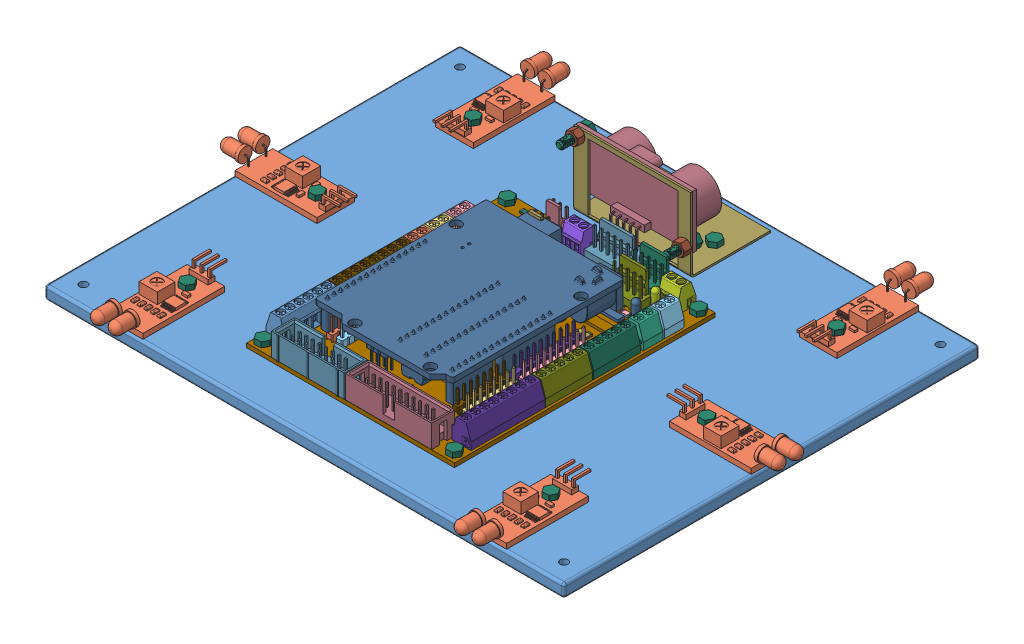
SolidWorks assembly upper assembly, configuration Default. Lengths in mm.
Overall size (215.6 59.56 175.6).
233 component instances, 198 part files, 38 mates.
Components (placement in the parent):
- base-1: base [Default] at (100.7293 111.0554 133.5181) size (200 5 160)
- Infrared Sensor (2)-1: Infrared Sensor (2) [Default] at (30.7293 116.0554 197.1202) x (-1 0 0) z (0 0 -1) size (14.5 8.55 44.7)
- Arduino Uno shield with Unokk-1: Arduino Uno shield with Unokk [Standard] at (60.7243 116.0554 95.3431) x (0 0 1) z (0 1 0) size (100.65 90.35 23.92)
  - PPP5f08ec48b7509.stp-1: PPP5f08ec48b7509.stp [Standard] at origin size (100.65 80.01 15.26)
    - CAPRR500W50L750T250H650P002.stp-1: CAPRR500W50L750T250H650P002.stp [Standard] at (21.59 34.29 1.57) x (0 -1 0) z (0 0 1) size (7.5 2.5 6.5)
    - CAPRR500W50L750T250H650P001.stp-1: CAPRR500W50L750T250H650P001.stp [Standard] at (21.59 34.29 1.57) x (0 -1 0) z (0 0 1) size (0.5 0.5 6.5)
    - CAPRR500W50L750T250H650P.stp-1: CAPRR500W50L750T250H650P.stp [Standard] at (21.59 34.29 1.57) x (0 -1 0) z (0 0 1) size (0.5 0.5 6.5)
    - CAPRR500W50L750T250H650P003.stp-1: CAPRR500W50L750T250H650P003.stp [Standard] at (20.32 26.67 1.57) x (0 -1 0) z (0 0 1) size (7.5 2.5 6.5)
    - CAPRR500W50L750T250H650P004.stp-1: CAPRR500W50L750T250H650P004.stp [Standard] at (20.32 26.67 1.57) x (0 -1 0) z (0 0 1) size (0.5 0.5 6.5)
    - CAPRR500W50L750T250H650P005.stp-1: CAPRR500W50L750T250H650P005.stp [Standard] at (20.32 26.67 1.57) x (0 -1 0) z (0 0 1) size (0.5 0.5 6.5)
    - Component_1.stp-1: Component_1.stp [Standard] at (26.67 60.325 1.57) x (0 1 0) z (0 0 1) size (15.24 3.56 1)
    - SW3dPS-MELF_Cylinder5.stp-1: SW3dPS-MELF_Cylinder5.stp [Standard] at (33.02 13.208 1.57) x (0 1 0) z (0 0 1) size (0.5 2.5 2.5)
    - SW3dPS-MELF_Cylinder7.stp-1: SW3dPS-MELF_Cylinder7.stp [Standard] at (33.02 13.208 1.57) x (0 1 0) z (0 0 1) size (0.8 2.5 2.5)
    - SW3dPS-MELF_Board1.stp-1: SW3dPS-MELF_Board1.stp [Standard] at (33.02 13.208 1.57) x (0 1 0) z (0 0 1) size (1.7 0.01 0.01)
    - SW3dPS-MELF_Cylinder9.stp-1: SW3dPS-MELF_Cylinder9.stp [Standard] at (33.02 13.208 1.57) x (0 1 0) z (0 0 1) size (2.4 2.5 2.5)
    - SW3dPS-MELF_Cylinder8.stp-1: SW3dPS-MELF_Cylinder8.stp [Standard] at (33.02 13.208 1.57) x (0 1 0) z (0 0 1) size (0.5 2.5 2.5)
    - SW3dPS-MELF_Cylinder6.stp-1: SW3dPS-MELF_Cylinder6.stp [Standard] at (33.02 13.208 1.57) x (0 1 0) z (0 0 1) size (0.8 2.5 2.5)
    - SW3dPS-MELF_Cylinder010.stp-1: SW3dPS-MELF_Cylinder010.stp [Standard] at (41.275 13.208 1.57) x (0 1 0) z (0 0 1) size (0.5 2.5 2.5)
    - SW3dPS-MELF_Cylinder011.stp-1: SW3dPS-MELF_Cylinder011.stp [Standard] at (41.275 13.208 1.57) x (0 1 0) z (0 0 1) size (0.8 2.5 2.5)
    - SW3dPS-MELF_Board002.stp-1: SW3dPS-MELF_Board002.stp [Standard] at (41.275 13.208 1.57) x (0 1 0) z (0 0 1) size (1.7 0.01 0.01)
    - SW3dPS-MELF_Cylinder012.stp-1: SW3dPS-MELF_Cylinder012.stp [Standard] at (41.275 13.208 1.57) x (0 1 0) z (0 0 1) size (2.4 2.5 2.5)
    - SW3dPS-MELF_Cylinder013.stp-1: SW3dPS-MELF_Cylinder013.stp [Standard] at (41.275 13.208 1.57) x (0 1 0) z (0 0 1) size (0.5 2.5 2.5)
    - SW3dPS-MELF_Cylinder014.stp-1: SW3dPS-MELF_Cylinder014.stp [Standard] at (41.275 13.208 1.57) x (0 1 0) z (0 0 1) size (0.8 2.5 2.5)
    - SW3dPS-MELF_Cylinder015.stp-1: SW3dPS-MELF_Cylinder015.stp [Standard] at (24.765 13.208 1.57) x (0 1 0) z (0 0 1) size (0.5 2.5 2.5)
    - SW3dPS-MELF_Cylinder016.stp-1: SW3dPS-MELF_Cylinder016.stp [Standard] at (24.765 13.208 1.57) x (0 1 0) z (0 0 1) size (0.8 2.5 2.5)
    - SW3dPS-MELF_Board003.stp-1: SW3dPS-MELF_Board003.stp [Standard] at (24.765 13.208 1.57) x (0 1 0) z (0 0 1) size (1.7 0.01 0.01)
    - SW3dPS-MELF_Cylinder017.stp-1: SW3dPS-MELF_Cylinder017.stp [Standard] at (24.765 13.208 1.57) x (0 1 0) z (0 0 1) size (2.4 2.5 2.5)
    - SW3dPS-MELF_Cylinder018.stp-1: SW3dPS-MELF_Cylinder018.stp [Standard] at (24.765 13.208 1.57) x (0 1 0) z (0 0 1) size (0.5 2.5 2.5)
    - SW3dPS-MELF_Cylinder019.stp-1: SW3dPS-MELF_Cylinder019.stp [Standard] at (24.765 13.208 1.57) x (0 1 0) z (0 0 1) size (0.8 2.5 2.5)
    - Component_2.stp-1: Component_2.stp [Standard] at (20.955 59.69 1.57) x (0 -1 0) z (0 0 1) size (10.16 2.54 1)
    - Component_3.stp-1: Component_3.stp [Standard] at (20.32 43.815 1.57) x (-1 0 0) z (0 0 1) size (10.16 3.17 1)
    - =_[0_1_1_2].stp-1: =_[0_1_1_2].stp [Standard] at (10.795 24.13 1.57) x (0 -1 0) z (0 0 1) size (7.62 5.8 15.26)
    - =_[0_1_1_2]001.stp-1: =_[0_1_1_2]001.stp [Standard] at (3.81 24.13 1.57) x (0 -1 0) z (0 0 1) size (7.62 5.8 15.26)
    - =_[0_1_1_2]002.stp-1: =_[0_1_1_2]002.stp [Standard] at (4.445 44.45 1.57) x (0 1 0) z (0 0 1) size (15.24 5.8 15.26)
    - =_[0_1_1_2]003.stp-1: =_[0_1_1_2]003.stp [Standard] at (4.699 59.055 1.57) x (0 1 0) z (0 0 1) size (12.7 5.8 15.26)
    - =_[0_1_1_2]004.stp-1: =_[0_1_1_2]004.stp [Standard] at (12.7 59.055 1.57) x (0 1 0) z (0 0 1) size (12.7 5.8 15.26)
    - 1.stp-1: 1.stp [Standard] at (49.276 63.5 1.57) x (-1 0 0) z (0 0 1) size (25.4 2.5 11.2)
    - 1001.stp-1: 1001.stp [Standard] at (73.66 63.5 1.57) x (-1 0 0) z (0 0 1) size (20.32 2.5 11.2)
    - 1002.stp-1: 1002.stp [Standard] at (55.88 15.24 1.57) x (-1 0 0) z (0 0 1) size (20.32 2.5 11.2)
    - 1003.stp-1: 1003.stp [Standard] at (76.2 15.24 1.57) size (15.24 2.5 11.2)
    - 1004.stp-1: 1004.stp [Standard] at (73.66 67.31 1.57) x (-1 0 0) z (0 0 1) size (20.32 2.5 11.2)
    - 1005.stp-1: 1005.stp [Standard] at (49.276 67.31 1.57) x (-1 0 0) z (0 0 1) size (25.4 2.5 11.2)
    - 1006.stp-1: 1006.stp [Standard] at (76.2 19.05 1.57) size (15.24 2.5 11.2)
    - 1007.stp-1: 1007.stp [Standard] at (55.88 19.05 1.57) x (-1 0 0) z (0 0 1) size (20.32 2.5 11.2)
    - LEDRD254W000D310H620P002.stp-1: LEDRD254W000D310H620P002.stp [Standard] at (12.065 69.215 1.57) x (0 1 0) z (0 0 1) size (3.1 3.1 6.2)
    - LEDRD254W000D310H620P.stp-1: LEDRD254W000D310H620P.stp [Standard] at (12.065 69.215 1.57) x (0 1 0) z (0 0 1) size (0.38 0.38 6.2)
    - LEDRD254W000D310H620P001.stp-1: LEDRD254W000D310H620P001.stp [Standard] at (12.065 69.215 1.57) x (0 1 0) z (0 0 1) size (0.38 0.38 6.2)
    - LEDRD254W000D310H620P003.stp-1: LEDRD254W000D310H620P003.stp [Standard] at (19.685 69.215 1.57) x (0 1 0) z (0 0 1) size (3.1 3.1 6.2)
    - LEDRD254W000D310H620P004.stp-1: LEDRD254W000D310H620P004.stp [Standard] at (19.685 69.215 1.57) x (0 1 0) z (0 0 1) size (0.38 0.38 6.2)
    - LEDRD254W000D310H620P005.stp-1: LEDRD254W000D310H620P005.stp [Standard] at (19.685 69.215 1.57) x (0 1 0) z (0 0 1) size (0.38 0.38 6.2)
    - LEDRD254W000D310H620P006.stp-1: LEDRD254W000D310H620P006.stp [Standard] at (50.8 52.705 1.57) x (-1 0 0) z (0 0 1) size (3.1 3.1 6.2)
    - LEDRD254W000D310H620P007.stp-1: LEDRD254W000D310H620P007.stp [Standard] at (50.8 52.705 1.57) x (-1 0 0) z (0 0 1) size (0.38 0.38 6.2)
    - LEDRD254W000D310H620P008.stp-1: LEDRD254W000D310H620P008.stp [Standard] at (50.8 52.705 1.57) x (-1 0 0) z (0 0 1) size (0.38 0.38 6.2)
    - LEDRD254W000D310H620P009.stp-1: LEDRD254W000D310H620P009.stp [Standard] at (45.72 52.705 1.57) x (-1 0 0) z (0 0 1) size (3.1 3.1 6.2)
    - LEDRD254W000D310H620P010.stp-1: LEDRD254W000D310H620P010.stp [Standard] at (45.72 52.705 1.57) x (-1 0 0) z (0 0 1) size (0.38 0.38 6.2)
    - LEDRD254W000D310H620P011.stp-1: LEDRD254W000D310H620P011.stp [Standard] at (45.72 52.705 1.57) x (-1 0 0) z (0 0 1) size (0.38 0.38 6.2)
    - User_Library-TO263-3New_Extruded_2.stp-1: User_Library-TO263-3New_Extruded_2.stp [Standard] at (41.91 31.75 1.57) x (-1 0 0) z (0 0 1) size (1.4 1.53 0.51)
    - User_Library-TO263-3New_Extruded.stp-1: User_Library-TO263-3New_Extruded.stp [Standard] at (41.91 31.75 1.57) x (-1 0 0) z (0 0 1) size (1 5.77 3.36)
    - User_Library-TO263-3New_D2PACK.stp-1: User_Library-TO263-3New_D2PACK.stp [Standard] at (41.91 31.75 1.57) x (-1 0 0) z (0 0 1) size (10.41 15.85 4.61)
    - User_Library-TO263-3New_Extruded_003.stp-1: User_Library-TO263-3New_Extruded_003.stp [Standard] at (54.61 31.75 1.57) x (-1 0 0) z (0 0 1) size (1.4 1.53 0.51)
    - User_Library-TO263-3New_Extruded001.stp-1: User_Library-TO263-3New_Extruded001.stp [Standard] at (54.61 31.75 1.57) x (-1 0 0) z (0 0 1) size (1 5.77 3.36)
    - User_Library-TO263-3New_D2PACK001.stp-1: User_Library-TO263-3New_D2PACK001.stp [Standard] at (54.61 31.75 1.57) x (-1 0 0) z (0 0 1) size (10.41 15.85 4.61)
    - User_Library-TO263-3New_Extruded_004.stp-1: User_Library-TO263-3New_Extruded_004.stp [Standard] at (29.21 31.75 1.57) x (-1 0 0) z (0 0 1) size (1.4 1.53 0.51)
    - User_Library-TO263-3New_Extruded002.stp-1: User_Library-TO263-3New_Extruded002.stp [Standard] at (29.21 31.75 1.57) x (-1 0 0) z (0 0 1) size (1 5.77 3.36)
    - User_Library-TO263-3New_D2PACK002.stp-1: User_Library-TO263-3New_D2PACK002.stp [Standard] at (29.21 31.75 1.57) x (-1 0 0) z (0 0 1) size (10.41 15.85 4.61)
    - RESC3216X078.stp-1: RESC3216X078.stp [Standard] at (54.483 46.482 1.57) size (2.12 1.6 0.1)
    - RESC3216X079.stp-1: RESC3216X079.stp [Standard] at (54.483 46.482 1.57) size (3.06 1.6 0.56)
    - RESC3216X077.stp-1: RESC3216X077.stp [Standard] at (54.483 46.482 1.57) size (0.57 1.6 0.76)
    - RESC3216X080.stp-1: RESC3216X080.stp [Standard] at (54.483 46.482 1.57) size (2.12 1.6 0.1)
    - RESC3216X76.stp-1: RESC3216X76.stp [Standard] at (54.483 46.482 1.57) size (0.57 1.6 0.76)
    - RESC3216X081.stp-1: RESC3216X081.stp [Standard] at (41.91 46.355 1.57) size (2.12 1.6 0.1)
    - RESC3216X082.stp-1: RESC3216X082.stp [Standard] at (41.91 46.355 1.57) size (3.06 1.6 0.56)
    - RESC3216X083.stp-1: RESC3216X083.stp [Standard] at (41.91 46.355 1.57) size (0.57 1.6 0.76)
    - RESC3216X084.stp-1: RESC3216X084.stp [Standard] at (41.91 46.355 1.57) size (2.12 1.6 0.1)
    - RESC3216X085.stp-1: RESC3216X085.stp [Standard] at (41.91 46.355 1.57) size (0.57 1.6 0.76)
    - RESC3216X086.stp-1: RESC3216X086.stp [Standard] at (29.21 48.895 1.57) size (2.12 1.6 0.1)
    - RESC3216X087.stp-1: RESC3216X087.stp [Standard] at (29.21 48.895 1.57) size (3.06 1.6 0.56)
    - RESC3216X088.stp-1: RESC3216X088.stp [Standard] at (29.21 48.895 1.57) size (0.57 1.6 0.76)
    - RESC3216X089.stp-1: RESC3216X089.stp [Standard] at (29.21 48.895 1.57) size (2.12 1.6 0.1)
    - RESC3216X090.stp-1: RESC3216X090.stp [Standard] at (29.21 48.895 1.57) size (0.57 1.6 0.76)
    - RESC3216X091.stp-1: RESC3216X091.stp [Standard] at (33.02 60.96 1.57) size (2.12 1.6 0.1)
    - RESC3216X092.stp-1: RESC3216X092.stp [Standard] at (33.02 60.96 1.57) size (3.06 1.6 0.56)
    - RESC3216X093.stp-1: RESC3216X093.stp [Standard] at (33.02 60.96 1.57) size (0.57 1.6 0.76)
    - RESC3216X094.stp-1: RESC3216X094.stp [Standard] at (33.02 60.96 1.57) size (2.12 1.6 0.1)
    - RESC3216X095.stp-1: RESC3216X095.stp [Standard] at (33.02 60.96 1.57) size (0.57 1.6 0.76)
    - RESC3216X096.stp-1: RESC3216X096.stp [Standard] at (33.02 63.5 1.57) size (2.12 1.6 0.1)
    - RESC3216X097.stp-1: RESC3216X097.stp [Standard] at (33.02 63.5 1.57) size (3.06 1.6 0.56)
    - RESC3216X098.stp-1: RESC3216X098.stp [Standard] at (33.02 63.5 1.57) size (0.57 1.6 0.76)
    - RESC3216X099.stp-1: RESC3216X099.stp [Standard] at (33.02 63.5 1.57) size (2.12 1.6 0.1)
    - RESC3216X100.stp-1: RESC3216X100.stp [Standard] at (33.02 63.5 1.57) size (0.57 1.6 0.76)
    - RESC3216X101.stp-1: RESC3216X101.stp [Standard] at (15.875 69.215 1.57) x (0 -1 0) z (0 0 1) size (2.12 1.6 0.1)
    - RESC3216X102.stp-1: RESC3216X102.stp [Standard] at (15.875 69.215 1.57) x (0 -1 0) z (0 0 1) size (3.06 1.6 0.56)
    - RESC3216X103.stp-1: RESC3216X103.stp [Standard] at (15.875 69.215 1.57) x (0 -1 0) z (0 0 1) size (0.57 1.6 0.76)
    - RESC3216X104.stp-1: RESC3216X104.stp [Standard] at (15.875 69.215 1.57) x (0 -1 0) z (0 0 1) size (2.12 1.6 0.1)
    - RESC3216X105.stp-1: RESC3216X105.stp [Standard] at (15.875 69.215 1.57) x (0 -1 0) z (0 0 1) size (0.57 1.6 0.76)
    - RESC3216X106.stp-1: RESC3216X106.stp [Standard] at (17.907 63.627 1.57) x (0 1 0) z (0 0 1) size (2.12 1.6 0.1)
    - RESC3216X107.stp-1: RESC3216X107.stp [Standard] at (17.907 63.627 1.57) x (0 1 0) z (0 0 1) size (3.06 1.6 0.56)
    - RESC3216X108.stp-1: RESC3216X108.stp [Standard] at (17.907 63.627 1.57) x (0 1 0) z (0 0 1) size (0.57 1.6 0.76)
    - RESC3216X109.stp-1: RESC3216X109.stp [Standard] at (17.907 63.627 1.57) x (0 1 0) z (0 0 1) size (2.12 1.6 0.1)
    - RESC3216X110.stp-1: RESC3216X110.stp [Standard] at (17.907 63.627 1.57) x (0 1 0) z (0 0 1) size (0.57 1.6 0.76)
    - RESC3216X111.stp-1: RESC3216X111.stp [Standard] at (50.673 57.023 1.57) x (-1 0 0) z (0 0 1) size (2.12 1.6 0.1)
    - RESC3216X112.stp-1: RESC3216X112.stp [Standard] at (50.673 57.023 1.57) x (-1 0 0) z (0 0 1) size (3.06 1.6 0.56)
    - RESC3216X113.stp-1: RESC3216X113.stp [Standard] at (50.673 57.023 1.57) x (-1 0 0) z (0 0 1) size (0.57 1.6 0.76)
    - RESC3216X114.stp-1: RESC3216X114.stp [Standard] at (50.673 57.023 1.57) x (-1 0 0) z (0 0 1) size (2.12 1.6 0.1)
    - RESC3216X115.stp-1: RESC3216X115.stp [Standard] at (50.673 57.023 1.57) x (-1 0 0) z (0 0 1) size (0.57 1.6 0.76)
    - RESC3216X116.stp-1: RESC3216X116.stp [Standard] at (46.99 57.277 1.57) x (0 -1 0) z (0 0 1) size (2.12 1.6 0.1)
    - RESC3216X117.stp-1: RESC3216X117.stp [Standard] at (46.99 57.277 1.57) x (0 -1 0) z (0 0 1) size (3.06 1.6 0.56)
    - RESC3216X118.stp-1: RESC3216X118.stp [Standard] at (46.99 57.277 1.57) x (0 -1 0) z (0 0 1) size (0.57 1.6 0.76)
    - RESC3216X119.stp-1: RESC3216X119.stp [Standard] at (46.99 57.277 1.57) x (0 -1 0) z (0 0 1) size (2.12 1.6 0.1)
    - RESC3216X120.stp-1: RESC3216X120.stp [Standard] at (46.99 57.277 1.57) x (0 -1 0) z (0 0 1) size (0.57 1.6 0.76)
    - RESC3216X121.stp-1: RESC3216X121.stp [Standard] at (34.925 45.085 1.57) x (-1 0 0) z (0 0 1) size (2.12 1.6 0.1)
    - RESC3216X122.stp-1: RESC3216X122.stp [Standard] at (34.925 45.085 1.57) x (-1 0 0) z (0 0 1) size (3.06 1.6 0.56)
    - RESC3216X123.stp-1: RESC3216X123.stp [Standard] at (34.925 45.085 1.57) x (-1 0 0) z (0 0 1) size (0.57 1.6 0.76)
    - RESC3216X124.stp-1: RESC3216X124.stp [Standard] at (34.925 45.085 1.57) x (-1 0 0) z (0 0 1) size (2.12 1.6 0.1)
    - RESC3216X125.stp-1: RESC3216X125.stp [Standard] at (34.925 45.085 1.57) x (-1 0 0) z (0 0 1) size (0.57 1.6 0.76)
    - RESC3216X126.stp-1: RESC3216X126.stp [Standard] at (47.625 46.101 1.57) x (0 -1 0) z (0 0 1) size (2.12 1.6 0.1)
    - RESC3216X127.stp-1: RESC3216X127.stp [Standard] at (47.625 46.101 1.57) x (0 -1 0) z (0 0 1) size (3.06 1.6 0.56)
    - RESC3216X128.stp-1: RESC3216X128.stp [Standard] at (47.625 46.101 1.57) x (0 -1 0) z (0 0 1) size (0.57 1.6 0.76)
    - RESC3216X129.stp-1: RESC3216X129.stp [Standard] at (47.625 46.101 1.57) x (0 -1 0) z (0 0 1) size (2.12 1.6 0.1)
    - RESC3216X130.stp-1: RESC3216X130.stp [Standard] at (47.625 46.101 1.57) x (0 -1 0) z (0 0 1) size (0.57 1.6 0.76)
    - RESC3216X131.stp-1: RESC3216X131.stp [Standard] at (59.69 48.006 1.57) x (0 -1 0) z (0 0 1) size (2.12 1.6 0.1)
    - RESC3216X132.stp-1: RESC3216X132.stp [Standard] at (59.69 48.006 1.57) x (0 -1 0) z (0 0 1) size (3.06 1.6 0.56)
    - RESC3216X133.stp-1: RESC3216X133.stp [Standard] at (59.69 48.006 1.57) x (0 -1 0) z (0 0 1) size (0.57 1.6 0.76)
    - RESC3216X134.stp-1: RESC3216X134.stp [Standard] at (59.69 48.006 1.57) x (0 -1 0) z (0 0 1) size (2.12 1.6 0.1)
    - RESC3216X135.stp-1: RESC3216X135.stp [Standard] at (59.69 48.006 1.57) x (0 -1 0) z (0 0 1) size (0.57 1.6 0.76)
    - RESC2012X072.stp-1: RESC2012X072.stp [Standard] at (10.795 50.165 1.57) x (-1 0 0) z (0 0 1) size (1.2 1.25 0.1)
    - RESC2012X073.stp-1: RESC2012X073.stp [Standard] at (10.795 50.165 1.57) x (-1 0 0) z (0 0 1) size (1.8 1.25 0.5)
    - RESC2012X071.stp-1: RESC2012X071.stp [Standard] at (10.795 50.165 1.57) x (-1 0 0) z (0 0 1) size (0.4 1.25 0.7)
    - RESC2012X074.stp-1: RESC2012X074.stp [Standard] at (10.795 50.165 1.57) x (-1 0 0) z (0 0 1) size (1.2 1.25 0.1)
    - RESC2012X70.stp-1: RESC2012X70.stp [Standard] at (10.795 50.165 1.57) x (-1 0 0) z (0 0 1) size (0.4 1.25 0.7)
    - RESC2012X075.stp-1: RESC2012X075.stp [Standard] at (10.795 47.625 1.57) x (-1 0 0) z (0 0 1) size (1.2 1.25 0.1)
    - RESC2012X076.stp-1: RESC2012X076.stp [Standard] at (10.795 47.625 1.57) x (-1 0 0) z (0 0 1) size (1.8 1.25 0.5)
    - RESC2012X077.stp-1: RESC2012X077.stp [Standard] at (10.795 47.625 1.57) x (-1 0 0) z (0 0 1) size (0.4 1.25 0.7)
    - RESC2012X078.stp-1: RESC2012X078.stp [Standard] at (10.795 47.625 1.57) x (-1 0 0) z (0 0 1) size (1.2 1.25 0.1)
    - RESC2012X079.stp-1: RESC2012X079.stp [Standard] at (10.795 47.625 1.57) x (-1 0 0) z (0 0 1) size (0.4 1.25 0.7)
    - RESC2012X080.stp-1: RESC2012X080.stp [Standard] at (10.795 45.085 1.57) x (-1 0 0) z (0 0 1) size (1.2 1.25 0.1)
    - RESC2012X081.stp-1: RESC2012X081.stp [Standard] at (10.795 45.085 1.57) x (-1 0 0) z (0 0 1) size (1.8 1.25 0.5)
    - RESC2012X082.stp-1: RESC2012X082.stp [Standard] at (10.795 45.085 1.57) x (-1 0 0) z (0 0 1) size (0.4 1.25 0.7)
    - RESC2012X083.stp-1: RESC2012X083.stp [Standard] at (10.795 45.085 1.57) x (-1 0 0) z (0 0 1) size (1.2 1.25 0.1)
    - RESC2012X084.stp-1: RESC2012X084.stp [Standard] at (10.795 45.085 1.57) x (-1 0 0) z (0 0 1) size (0.4 1.25 0.7)
    - RESC2012X085.stp-1: RESC2012X085.stp [Standard] at (10.795 42.545 1.57) x (-1 0 0) z (0 0 1) size (1.2 1.25 0.1)
    - RESC2012X086.stp-1: RESC2012X086.stp [Standard] at (10.795 42.545 1.57) x (-1 0 0) z (0 0 1) size (1.8 1.25 0.5)
    - RESC2012X087.stp-1: RESC2012X087.stp [Standard] at (10.795 42.545 1.57) x (-1 0 0) z (0 0 1) size (0.4 1.25 0.7)
    - RESC2012X088.stp-1: RESC2012X088.stp [Standard] at (10.795 42.545 1.57) x (-1 0 0) z (0 0 1) size (1.2 1.25 0.1)
    - RESC2012X089.stp-1: RESC2012X089.stp [Standard] at (10.795 42.545 1.57) x (-1 0 0) z (0 0 1) size (0.4 1.25 0.7)
    - RESC2012X090.stp-1: RESC2012X090.stp [Standard] at (10.795 40.005 1.57) x (-1 0 0) z (0 0 1) size (1.2 1.25 0.1)
    - RESC2012X091.stp-1: RESC2012X091.stp [Standard] at (10.795 40.005 1.57) x (-1 0 0) z (0 0 1) size (1.8 1.25 0.5)
    - RESC2012X092.stp-1: RESC2012X092.stp [Standard] at (10.795 40.005 1.57) x (-1 0 0) z (0 0 1) size (0.4 1.25 0.7)
    - RESC2012X093.stp-1: RESC2012X093.stp [Standard] at (10.795 40.005 1.57) x (-1 0 0) z (0 0 1) size (1.2 1.25 0.1)
    - RESC2012X094.stp-1: RESC2012X094.stp [Standard] at (10.795 40.005 1.57) x (-1 0 0) z (0 0 1) size (0.4 1.25 0.7)
    - RESC2012X095.stp-1: RESC2012X095.stp [Standard] at (10.795 37.465 1.57) x (-1 0 0) z (0 0 1) size (1.2 1.25 0.1)
    - RESC2012X096.stp-1: RESC2012X096.stp [Standard] at (10.795 37.465 1.57) x (-1 0 0) z (0 0 1) size (1.8 1.25 0.5)
    - RESC2012X097.stp-1: RESC2012X097.stp [Standard] at (10.795 37.465 1.57) x (-1 0 0) z (0 0 1) size (0.4 1.25 0.7)
    - RESC2012X098.stp-1: RESC2012X098.stp [Standard] at (10.795 37.465 1.57) x (-1 0 0) z (0 0 1) size (1.2 1.25 0.1)
    - RESC2012X099.stp-1: RESC2012X099.stp [Standard] at (10.795 37.465 1.57) x (-1 0 0) z (0 0 1) size (0.4 1.25 0.7)
    - RESC3216X136.stp-1: RESC3216X136.stp [Standard] at (64.135 32.639 1.57) x (0 1 0) z (0 0 1) size (2.12 1.6 0.1)
    - RESC3216X137.stp-1: RESC3216X137.stp [Standard] at (64.135 32.639 1.57) x (0 1 0) z (0 0 1) size (3.06 1.6 0.56)
    - RESC3216X138.stp-1: RESC3216X138.stp [Standard] at (64.135 32.639 1.57) x (0 1 0) z (0 0 1) size (0.57 1.6 0.76)
    - RESC3216X139.stp-1: RESC3216X139.stp [Standard] at (64.135 32.639 1.57) x (0 1 0) z (0 0 1) size (2.12 1.6 0.1)
    - RESC3216X140.stp-1: RESC3216X140.stp [Standard] at (64.135 32.639 1.57) x (0 1 0) z (0 0 1) size (0.57 1.6 0.76)
    - RESC3216X141.stp-1: RESC3216X141.stp [Standard] at (3.683 10.795 1.57) x (0 1 0) z (0 0 1) size (2.12 1.6 0.1)
    - RESC3216X142.stp-1: RESC3216X142.stp [Standard] at (3.683 10.795 1.57) x (0 1 0) z (0 0 1) size (3.06 1.6 0.56)
    - RESC3216X143.stp-1: RESC3216X143.stp [Standard] at (3.683 10.795 1.57) x (0 1 0) z (0 0 1) size (0.57 1.6 0.76)
    - RESC3216X144.stp-1: RESC3216X144.stp [Standard] at (3.683 10.795 1.57) x (0 1 0) z (0 0 1) size (2.12 1.6 0.1)
    - RESC3216X145.stp-1: RESC3216X145.stp [Standard] at (3.683 10.795 1.57) x (0 1 0) z (0 0 1) size (0.57 1.6 0.76)
    - RESC3216X146.stp-1: RESC3216X146.stp [Standard] at (74.422 51.943 1.57) x (0 -1 0) z (0 0 1) size (2.12 1.6 0.1)
    - RESC3216X147.stp-1: RESC3216X147.stp [Standard] at (74.422 51.943 1.57) x (0 -1 0) z (0 0 1) size (3.06 1.6 0.56)
    - RESC3216X148.stp-1: RESC3216X148.stp [Standard] at (74.422 51.943 1.57) x (0 -1 0) z (0 0 1) size (0.57 1.6 0.76)
    - RESC3216X149.stp-1: RESC3216X149.stp [Standard] at (74.422 51.943 1.57) x (0 -1 0) z (0 0 1) size (2.12 1.6 0.1)
    - RESC3216X150.stp-1: RESC3216X150.stp [Standard] at (74.422 51.943 1.57) x (0 -1 0) z (0 0 1) size (0.57 1.6 0.76)
    - RESC3216X151.stp-1: RESC3216X151.stp [Standard] at (3.683 17.272 1.57) x (0 1 0) z (0 0 1) size (2.12 1.6 0.1)
    - RESC3216X152.stp-1: RESC3216X152.stp [Standard] at (3.683 17.272 1.57) x (0 1 0) z (0 0 1) size (3.06 1.6 0.56)
    - RESC3216X153.stp-1: RESC3216X153.stp [Standard] at (3.683 17.272 1.57) x (0 1 0) z (0 0 1) size (0.57 1.6 0.76)
    - RESC3216X154.stp-1: RESC3216X154.stp [Standard] at (3.683 17.272 1.57) x (0 1 0) z (0 0 1) size (2.12 1.6 0.1)
    - RESC3216X155.stp-1: RESC3216X155.stp [Standard] at (3.683 17.272 1.57) x (0 1 0) z (0 0 1) size (0.57 1.6 0.76)
    - Component_4.stp-1: Component_4.stp [Standard] at (11.684 10.287 1.57) size (2 2 1)
    - User_Library-BH-10...64.stp-1: User_Library-BH-10...64.stp [Standard] at (95.885 54.61 1.57) x (0 1 0) z (0 0 1) size (33.06 9.2 12.14)
    - User_Library-BH-10...065.stp-1: User_Library-BH-10...065.stp [Standard] at (95.885 23.495 1.57) x (0 -1 0) z (0 0 1) size (27.98 9.2 12.14)
    - mkds_1-5-3.5_mkds_1-5-3.5;mkds_1-5-3.5.stp-1: mkds_1-5-3.5_mkds_1-5-3.5;mkds_1-5-3.5.stp [Standard] at (36.83 75.565 1.57) size (18 7.3 12)
    - mkds_1-5-3.5_mkds_1-5-3.5;mkds_1-5-3.006.stp-1: mkds_1-5-3.5_mkds_1-5-3.5;mkds_1-5-3.006.stp [Standard] at (55.245 75.565 1.57) size (18 7.3 12)
    - mkds_1-8-3.5_mkds_1-8-3.5;mkds_1-8-3.5.stp-1: mkds_1-8-3.5_mkds_1-8-3.5;mkds_1-8-3.5.stp [Standard] at (78.74 75.565 1.57) size (28.5 7.3 12)
    - mkds_1-8-3.5_mkds_1-8-3.5;mkds_1-8-3.006.stp-1: mkds_1-8-3.5_mkds_1-8-3.5;mkds_1-8-3.006.stp [Standard] at (57.785 4.445 1.57) x (-1 0 0) z (0 0 1) size (28.5 7.3 12)
    - mkds_1-6-3.5_mkds_1-6-3.5;mkds_1-6-3.5.stp-1: mkds_1-6-3.5_mkds_1-6-3.5;mkds_1-6-3.5.stp [Standard] at (83.185 4.445 1.57) x (-1 0 0) z (0 0 1) size (21.5 7.3 12)
    - mkds_1-2-3.5_mkds_1-2-3.5;mkds_1-2-3.5.stp-1: mkds_1-2-3.5_mkds_1-2-3.5;mkds_1-2-3.5.stp [Standard] at (39.37 4.445 1.57) x (-1 0 0) z (0 0 1) size (7.5 7.3 12)
    - mkds_1-2-3.5_mkds_1-2-3.5;mkds_1-2-3.006.stp-1: mkds_1-2-3.5_mkds_1-2-3.5;mkds_1-2-3.006.stp [Standard] at (31.115 4.445 1.57) x (-1 0 0) z (0 0 1) size (7.5 7.3 12)
    - mkds_1-2-3.5_mkds_1-2-3.5;mkds_1-2-3.007.stp-1: mkds_1-2-3.5_mkds_1-2-3.5;mkds_1-2-3.007.stp [Standard] at (22.86 4.445 1.57) x (-1 0 0) z (0 0 1) size (7.5 7.3 12)
    - mkds_1-2-3.5_mkds_1-2-3.5;mkds_1-2-3.008.stp-1: mkds_1-2-3.5_mkds_1-2-3.5;mkds_1-2-3.008.stp [Standard] at (14.605 75.565 1.57) size (7.5 7.3 12)
    - mkds_1-2-3.5_mkds_1-2-3.5;mkds_1-2-3.009.stp-1: mkds_1-2-3.5_mkds_1-2-3.5;mkds_1-2-3.009.stp [Standard] at (22.86 75.565 1.57) size (7.5 7.3 12)
    - mkds_1-2-3.5_mkds_1-2-3.5;mkds_1-2-3.010.stp-1: mkds_1-2-3.5_mkds_1-2-3.5;mkds_1-2-3.010.stp [Standard] at (4.445 69.85 1.57) x (0 1 0) z (0 0 1) size (7.5 7.3 12)
    - mkds_1-2-3.5_mkds_1-2-3.5;mkds_1-2-3.011.stp-1: mkds_1-2-3.5_mkds_1-2-3.5;mkds_1-2-3.011.stp [Standard] at (4.445 32.385 1.57) x (0 1 0) z (0 0 1) size (7.5 7.3 12)
    - Component_Component.stp-1: Component_Component.stp [Standard] at origin size (100.33 80.01 1.57)
  - arduino uno-2: arduino uno [Default] at (52.02 37.3929 14.21) x (1 0 0) z (0 1 0) size (76.5 14.6 53)
  - kkkkk-2: kkkkk [Default] at (132.8181 -85.8824 -60.2258) x (0.934285 0.356528 0) z (0 0 1) size (6.55 6.85 3.19)
    - Part3^kkkkk-1: Part3^kkkkk [Default] at origin (virtual)
    - Part2^kkkkk-1: Part2^kkkkk [Default] at origin (virtual)
    - nut (1) (1)-1: nut (1) (1) [Default] at (-59.1167 207.857 53.7136) x (0.966766 -0.255664 0) z (0 0 1) size (5.28 5.69 3.19)
- Part1^upper assembly-1: Part1^upper assembly [Default] at origin (virtual)
- ultrasonic base-1: ultrasonic base [Default] at (100.7293 116.792 86.5181) size (45 28.74 30.74)
- ULTRASONIC SENSOR-1: ULTRASONIC SENSOR [Default] at (100.7293 134.542 86.5181) x (-1 0 0) z (0 0 -1) size (45 26.75 17.75)
- Battery Pack-1: Battery Pack [Default] at (104.3003 111.0554 137.8439) x (-0.999864 0 -0.016497) z (0 -1 0) size (127.8 34 24)
- Infrared Sensor (2)-7: Infrared Sensor (2) [Default] at (17.1272 116.0554 133.5181) x (0 0 -1) z (1 0 0) size (14.5 8.55 44.7)
- nut (1) (1)-50: nut (1) (1) [Default] at (25.7293 109.5554 133.5181) x (1 0 0) z (0 1 0) size (5.28 5.69 3.19)
- bolt-1: bolt [Default] at (25.7293 119.0554 133.5181) x (1 0 0) z (0 -1 0) size (5.19 4.62 12)
- bolt-2: bolt [Default] at (116.7293 117.792 71.5181) x (-0.837169 0 -0.546944) z (0 -1 0) size (5.19 4.62 12)
- nut (1) (1)-51: nut (1) (1) [Default] at (116.7293 109.5554 71.5181) x (1 0 0) z (0 -1 0) size (5.28 5.69 3.19)
- bolt-3: bolt [Default] at (30.7293 119.0554 188.5181) x (1 0 0) z (0 -1 0) size (5.19 4.62 12)
- nut (1) (1)-52: nut (1) (1) [Default] at (30.7293 109.5554 188.5181) x (-0.016879 0 -0.999858) z (0 1 0) size (5.28 5.69 3.19)
- bolt-4: bolt [Default] at (63.8993 118.7805 98.5181) x (1 0 0) z (0 -1 0) size (5.19 4.62 12)
- nut (1) (1)-53: nut (1) (1) [Default] at (63.8993 109.5554 98.5181) x (0.573542 0 -0.819176) z (0 -1 0) size (5.28 5.69 3.19)
- bolt-5: bolt [Default] at (121.2293 126.292 84.0181) x (0.642048 -0.766665 0) z (0 0 1) size (5.19 4.62 12)
- nut (1) (1)-54: nut (1) (1) [Default] at (80.2293 142.792 88.7547) x (0.608509 -0.793547 0) z (0 0 1) size (5.28 5.69 3.19)
- bolt-6: bolt [Default] at (80.2293 142.792 84.0181) x (0.603765 -0.797163 0) z (0 0 1) size (5.19 4.62 12)
- nut (1) (1)-55: nut (1) (1) [Default] at (121.2293 126.292 88.7547) x (-0.383579 0.923508 0) z (0 0 1) size (5.28 5.69 3.19)
- bolt-7: bolt [Default] at (100.7293 117.792 71.5181) x (1 0 0) z (0 -1 0) size (5.19 4.62 12)
- nut (1) (1)-56: nut (1) (1) [Default] at (100.7293 109.5554 71.5181) x (1 0 0) z (0 -1 0) size (5.28 5.69 3.19)
- nut (1) (1)-57: nut (1) (1) [Default] at (137.5593 109.5554 98.5181) x (0.573542 0 0.819176) z (0 -1 0) size (5.28 5.69 3.19)
- bolt-8: bolt [Default] at (137.5593 118.7805 98.5181) x (-1 0 0) z (0 -1 0) size (5.19 4.62 12)
- nut (1) (1)-58: nut (1) (1) [Default] at (63.8993 109.5554 192.4981) x (-0.573542 0 -0.819176) z (0 -1 0) size (5.28 5.69 3.19)
- bolt-9: bolt [Default] at (63.8993 118.7805 192.4981) x (1 0 0) z (0 -1 0) size (5.19 4.62 12)
- nut (1) (1)-59: nut (1) (1) [Default] at (137.5593 109.5561 192.4981) x (0.573542 0 -0.819176) z (0 1 0) size (5.28 5.69 3.19)
- bolt-10: bolt [Default] at (137.5593 118.7805 192.4981) x (-1 0 0) z (0 -1 0) size (5.19 4.62 12)
- Infrared Sensor (2)-8: Infrared Sensor (2) [Default] at (184.3314 116.0554 133.5181) x (0 0 1) z (-1 0 0) size (14.5 8.55 44.7)
- bolt-11: bolt [Default] at (175.7293 119.0554 133.5181) x (-1 0 0) z (0 -1 0) size (5.19 4.62 12)
- nut (1) (1)-60: nut (1) (1) [Default] at (175.7293 109.5548 133.5181) x (-1 0 0) z (0 -1 0) size (5.28 5.69 3.19)
- Infrared Sensor (2)-9: Infrared Sensor (2) [Default] at (30.7293 116.0554 69.916) size (14.5 8.55 44.7)
- bolt-12: bolt [Default] at (30.7293 119.0554 78.5181) x (1 0 0) z (0 -1 0) size (5.19 4.62 12)
- nut (1) (1)-61: nut (1) (1) [Default] at (30.7293 109.5548 78.5181) x (-0.016879 0 0.999858) z (0 -1 0) size (5.28 5.69 3.19)
- Infrared Sensor (2)-10: Infrared Sensor (2) [Default] at (170.7293 116.0554 197.1202) x (-1 0 0) z (0 0 -1) size (14.5 8.55 44.7)
- bolt-13: bolt [Default] at (170.7293 119.0554 188.5181) x (1 0 0) z (0 -1 0) size (5.19 4.62 12)
- nut (1) (1)-62: nut (1) (1) [Default] at (170.7293 109.5554 188.5181) x (-0.016879 0 0.999858) z (0 1 0) size (5.28 5.69 3.19)
- Infrared Sensor (2)-11: Infrared Sensor (2) [Default] at (170.7293 116.0554 69.916) size (14.5 8.55 44.7)
- bolt-14: bolt [Default] at (170.7293 119.0554 78.5181) x (1 0 0) z (0 -1 0) size (5.19 4.62 12)
- nut (1) (1)-63: nut (1) (1) [Default] at (170.7293 109.5548 78.5181) x (-0.016879 0 -0.999858) z (0 -1 0) size (5.28 5.69 3.19)
Mates (geometry in assembly coordinates):
- Concentric5: concentric anti-aligned: circle of base-1; circle of Arduino Uno shield with Uno-1/PPP5f08ec48b7509.stp-1/Component_Component.stp-1
- Concentric6: concentric anti-aligned: circle of base-1; circle of Arduino Uno shield with Uno-1/PPP5f08ec48b7509.stp-1/Component_Component.stp-1
- Parallel1: parallel aligned: line of base-1 through (157.7163 116.0554 83.356) axis (0 -1 0); line of Arduino Uno shield with Unokk-1/kkkkk-2/nut-1 through (-52.7101 224.8507 158.6743) axis (0 -1 0)
- Parallel6: parallel aligned: line of base-1 through (63.8993 116.0554 98.5181) axis (0 -1 0); line of Arduino Uno shield with Unokk-1/kkkkk-2/nut-1 through (-52.7101 224.8507 158.6743) axis (0 -1 0)
- Parallel7: parallel aligned: line of base-1 through (63.8993 116.0554 98.5181) axis (0 -1 0); line of Arduino Uno shield with Unokk-1/kkkkk-2/nut-1 through (-52.7101 224.8507 158.6743) axis (0 -1 0)
- Coincident56: coincident anti-aligned: plane of base-1 through (100.7293 111.0554 133.5181) normal (0 -1 0); plane of Battery Pack-1 through (104.3003 111.0554 137.8439) normal (0 1 0)
- Coincident57: coincident anti-aligned: plane of base-1 through (100.7293 116.0554 133.5181) normal (0 1 0); plane of Arduino Uno shield with Unokk-1/PPP5f08ec48b7509.stp-1/Component_Component.stp-1 through (60.7243 116.0554 95.3431) normal (0 -1 0)
- Coincident61: coincident aligned: circle of base-1; circle of ultrasonic base-1
- Concentric16: concentric aligned: circle of ultrasonic base-1; circle of ULTRASONIC SENSOR-1
- Concentric17: concentric aligned: circle of ultrasonic base-1; circle of ULTRASONIC SENSOR-1
- Coincident81: coincident anti-aligned: plane of ultrasonic base-1 through (123.2293 116.792 86.5181) normal (0 0 -1); plane of ULTRASONIC SENSOR-1 through (100.7293 134.542 86.5181) normal (0 0 1)
- Coincident84: coincident anti-aligned: circle of base-1; circle of Infrared Sensor (2)-1
- Parallel8: parallel aligned: line of base-1 through (1.7293 116.0554 212.5181) axis (1 0 0); line of Infrared Sensor (2)-1 through (23.4793 116.0554 212.8702) axis (1 0 0)
- Coincident86: coincident anti-aligned: circle of base-1; circle of Infrared Sensor (2)-7
- Parallel11: parallel anti-aligned: line of base-1 through (0.7293 115.0554 212.5181) axis (0 0 -1); line of Infrared Sensor (2)-7 through (1.3772 116.0554 126.2681) axis (0 0 1)
- Coincident91: coincident anti-aligned: circle of Infrared Sensor (2)-7; circle of bolt-1
- Coincident92: coincident anti-aligned: circle of base-1; circle of nut (1) (1)-50
- Coincident93: coincident anti-aligned: circle of Infrared Sensor (2)-1; circle of bolt-3
- Coincident94: coincident anti-aligned: line of base-1 through (30.7293 116.0554 188.5181) axis (0 -1 0); line of nut (1) (1)-52 through (30.7293 110.2261 188.5181) axis (0 1 0)
- Coincident95: coincident anti-aligned: plane of base-1 through (100.7293 111.0554 133.5181) normal (0 -1 0); plane of nut (1) (1)-52 through (30.7293 111.0554 188.5181) normal (0 1 0)
- Concentric18: concentric anti-aligned: circle of Arduino Uno shield with Unokk-1/PPP5f08ec48b7509.stp-1/Component_Component.stp-1; circle of bolt-4
- Coincident96: coincident anti-aligned: line of bolt-4 through (63.8993 108.1452 98.5181) axis (0 -1 0); line of nut (1) (1)-53 through (63.8993 110.2417 98.5181) axis (0 1 0)
- Coincident97: coincident anti-aligned: plane of base-1 through (100.7293 111.0554 133.5181) normal (0 -1 0); plane of nut (1) (1)-53 through (63.8993 111.0554 98.5181) normal (0 1 0)
- Coincident98: coincident anti-aligned: line of ultrasonic base-1 through (80.2293 142.792 87.2547) axis (0 0 -1); line of nut (1) (1)-54 through (80.2293 142.792 89.4253) axis (0 0 1)
- Coincident99: coincident anti-aligned: plane of ultrasonic base-1 through (123.2293 116.792 87.2547) normal (0 0 1); plane of nut (1) (1)-54 through (80.2293 142.792 87.2547) normal (0 0 -1)
- Coincident100: coincident anti-aligned: line of ULTRASONIC SENSOR-1 through (121.2293 126.292 85.0181) axis (0 0 1); line of nut (1) (1)-55 through (121.2293 126.292 90.2547) axis (0 0 -1)
- Coincident102: coincident anti-aligned: plane of ultrasonic base-1 through (123.2293 116.792 87.2547) normal (0 0 1); plane of nut (1) (1)-55 through (121.2293 126.292 87.2547) normal (0 0 -1)
- Concentric20: concentric anti-aligned: circle of ULTRASONIC SENSOR-1; circle of bolt-6
- Coincident103: coincident: plane of ULTRASONIC SENSOR-1 through (100.7293 134.542 85.0181) normal (0 0 -1); line of bolt-6 through (81.3522 145.1349 85.0181) axis (-0.997065 -0.076558 0)
- Concentric21: concentric anti-aligned: circle of ULTRASONIC SENSOR-1; circle of bolt-5
- Coincident104: coincident: plane of ULTRASONIC SENSOR-1 through (100.7293 134.542 85.0181) normal (0 0 -1); line of bolt-5 through (122.7999 124.2225 85.0181) axis (0.387589 0.921832 0)
- Coincident105: coincident anti-aligned: circle of base-1; circle of ultrasonic base-1
- Coincident106: coincident anti-aligned: circle of ultrasonic base-1; circle of bolt-7
- Coincident107: coincident anti-aligned: line of base-1 through (100.7293 116.0554 71.5181) axis (0 -1 0); line of nut (1) (1)-56 through (100.7293 110.2417 71.5181) axis (0 1 0)
- Coincident109: coincident anti-aligned: plane of base-1 through (100.7293 111.0554 133.5181) normal (0 -1 0); plane of nut (1) (1)-56 through (100.7293 111.0554 71.5181) normal (0 1 0)
- Coincident110: coincident aligned: circle of ultrasonic base-1; circle of bolt-2
- Coincident111: coincident anti-aligned: line of base-1 through (116.7293 116.0554 71.5181) axis (0 -1 0); line of nut (1) (1)-51 through (116.7293 108.0554 71.5181) axis (0 1 0)
- Coincident112: coincident anti-aligned: plane of base-1 through (100.7293 111.0554 133.5181) normal (0 -1 0); plane of nut (1) (1)-51 through (116.7293 111.0554 71.5181) normal (0 1 0)
